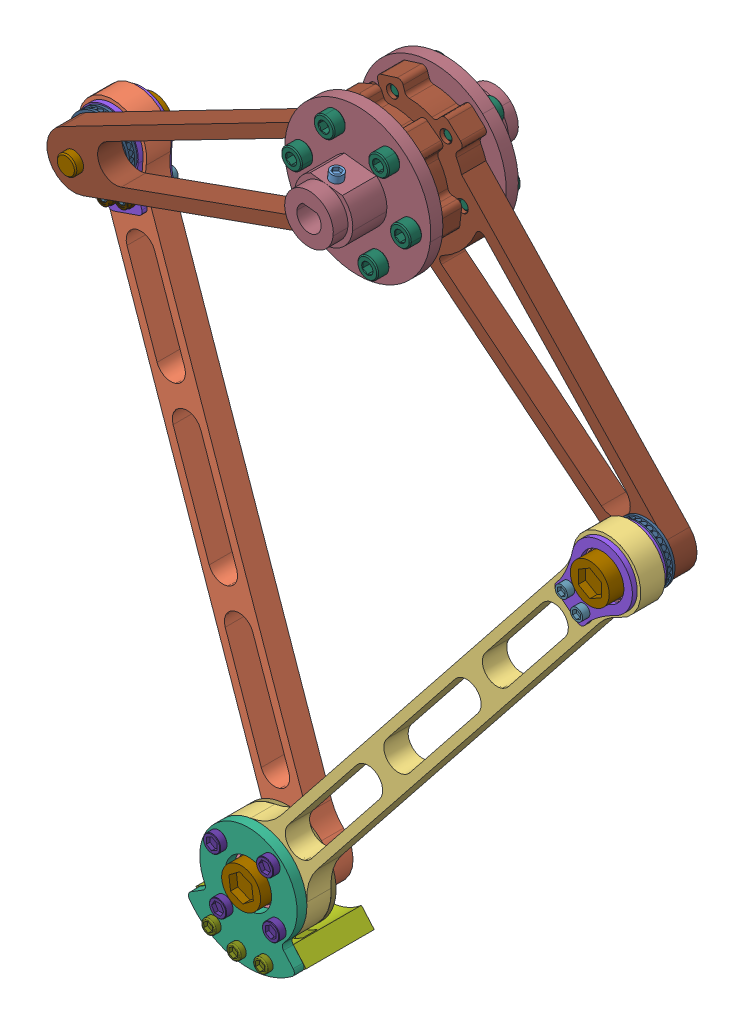
SolidWorks assembly B【部分装配】单腿, configuration 默认. Lengths in mm.
Overall size (272.8 367.82 76).
59 component instances, 19 part files, 123 mates.
Components (placement in the parent):
- 【光杆】M8-26-1: 【光杆】M8-26 [默认] at (-54.1395 107.9451 129.2539) x (0.99429 0.106711 0) z (0 0 1) size (8 8 26)
- 【铝合金结构件】小腿1-1: 【铝合金结构件】小腿1 [默认] at (-175.7689 55.1337 129.2539) x (0.329361 -0.944204 0) z (0 0 1) size (257 28 10)
- 【铝合金结构件】小腿2-1: 【铝合金结构件】小腿2 [默认] at (43.2186 17.9219 145.2539) x (-0.622759 -0.782414 0) z (0 0 1) size (264 40 10)
- 【深沟球轴承】6800ZZ 尺寸：10-19-5-3: 【深沟球轴承】6800ZZ 尺寸：10-19-5 [默认] at (43.2186 17.9219 145.2539) x (0.672447 0.740145 0) z (0 0 1) size (19 19 5)
- 【深沟球轴承】6800ZZ 尺寸：10-19-5-4: 【深沟球轴承】6800ZZ 尺寸：10-19-5 [默认] at (43.2186 17.9219 150.2539) x (1 0.000049 0) z (0 0 1) size (19 19 5)
- 【深沟球轴承】6800ZZ 尺寸：10-19-5-8: 【深沟球轴承】6800ZZ 尺寸：10-19-5 [默认] at (-175.7689 55.1337 134.2539) x (1 -0.000082 0) z (0 0 1) size (19 19 5)
- 【深沟球轴承】6800ZZ 尺寸：10-19-5-9: 【深沟球轴承】6800ZZ 尺寸：10-19-5 [默认] at (-175.7689 55.1337 129.2539) size (19 19 5)
- 【深沟球轴承】6800ZZ 尺寸：10-19-5-10: 【深沟球轴承】6800ZZ 尺寸：10-19-5 [默认] at (-100.016 -162.0332 150.2539) x (1 -0.000016 0) z (0 0 1) size (19 19 5)
- 【深沟球轴承】6800ZZ 尺寸：10-19-5-11: 【深沟球轴承】6800ZZ 尺寸：10-19-5 [默认] at (-100.016 -162.0332 145.2539) x (1 -0.00012 0) z (0 0 1) size (19 19 5)
- 【深沟球轴承】608ZZ 尺寸：8-22-7-3: 【深沟球轴承】608ZZ 尺寸：8-22-7 [Défaut] at (-54.1395 107.9451 151.7539) size (22 22 7)
- 【深沟球轴承】608ZZ 尺寸：8-22-7-4: 【深沟球轴承】608ZZ 尺寸：8-22-7 [Défaut] at (-54.1395 107.9451 132.6539) size (22 22 7)
- 【马蹄结构件】蹄子侧板-3: 【马蹄结构件】蹄子侧板 [默认] at (25.2358 10.7897 159.2539) x (-0.98897 0.148118 0) z (0 0 -1) size (43.97 50 4)
- 【马蹄结构件】蹄子底板-1: 【马蹄结构件】蹄子底板 [默认] at (-169.1792 40.0334 155.2539) x (0.98897 -0.148118 0) z (0 0 1) size (45.72 15.8 28)
- 【碳纤维板垫圈】15-23-1-1: 【碳纤维板垫圈】15-23-1 [默认] at (-175.7689 55.1337 128.2539) x (-0.329361 0.944204 0) z (0 0 1) size (35.5 25 2)
- 【碳纤维板垫圈】15-23-1-3: 【碳纤维板垫圈】15-23-1 [默认] at (-175.7689 55.1337 140.2539) x (-0.329361 0.944204 0) z (0 0 1) size (35.5 25 2)
- 【碳纤维板垫圈】15-23-1-4: 【碳纤维板垫圈】15-23-1 [默认] at (43.2186 17.9219 156.2539) x (0.622759 0.782414 0) z (0 0 1) size (35.5 25 2)
- 【碳纤维板垫圈】15-23-1-5: 【碳纤维板垫圈】15-23-1 [默认] at (43.2186 17.9219 144.2539) x (0.622759 0.782414 0) z (0 0 1) size (35.5 25 2)
- 【塞打螺丝】M10-16-8: 【塞打螺丝】M10-16 [默认] at (-175.7689 55.1337 145.2539) x (1 0 0) z (0 0 -1) size (16 16 36.25)
- 【平面推力滚针轴承】尺寸：10-24-4-7: 【平面推力滚针轴承】尺寸：10-24-4 [默认] at (-175.7689 55.1337 141.2539) size (24 24 4)
- 【铝合金结构件】大腿-6: 【铝合金结构件】大腿 [默认] at (-188.126 -167.5744 109.2539) x (0.744298 -0.667848 0) z (0 0 1) size (92.95 159.3 10)
- 【塞打螺丝】M10-16-9: 【塞打螺丝】M10-16 [默认] at (43.2186 17.9219 139.2539) size (16 16 36.25)
- 【平面推力滚针轴承】尺寸：10-24-4-8: 【平面推力滚针轴承】尺寸：10-24-4 [默认] at (43.2186 17.9219 139.2539) size (24 24 4)
- 【铝合金结构件】大腿-7: 【铝合金结构件】大腿 [默认] at (252.0136 96.3837 93.2539) x (0.311173 0.950353 0) z (0 0 1) size (92.95 159.3 10)
- 【碳纤维板垫圈】17-40-2-2: 【碳纤维板垫圈】17-40-2 [默认] at (-100.016 -162.0332 143.2539) x (0.622759 0.782414 0) z (0 0 1) size (40 40 2)
- 【平面推力滚针轴承】尺寸：10-24-4-9: 【平面推力滚针轴承】尺寸：10-24-4 [默认] at (-100.016 -162.0332 139.2539) size (24 24 4)
- 【塞打螺丝】M10-16-10: 【塞打螺丝】M10-16 [默认] at (-100.016 -162.0332 139.2539) x (-0.606643 0.794975 0) z (0 0 1) size (16 16 36.25)
- 【法兰联轴器】M10-孔3-1: 【法兰联轴器】M10-孔3 [默认] at (-17.0813 108.8956 37.7039) x (0.999235 0.039114 0) z (0 0 1) size (84.85 84.85 25)
  - 3508__________.STEP-1: 3508__________.STEP [默认] at (-37.067 0.4997 66.55) x (-0.707107 -0.707107 0) z (0 0 1) size (60 60 25)
- 【法兰联轴器】M10-孔3-2: 【法兰联轴器】M10-孔3 [默认] at (-82.8494 84.4941 246.8039) x (-0.78293 -0.62211 0) z (0 0 -1) size (84.85 84.85 25)
  - 3508__________.STEP-1: 3508__________.STEP [默认] at (-37.067 0.4997 66.55) x (-0.707107 -0.707107 0) z (0 0 1) size (60 60 25)
- 【螺丝】M3-18 杯头内六角-1: 【螺丝】M3-18 杯头内六角 [默认] at (-173.9466 37.7648 145.2539) x (-1 0 0) z (0 0 -1) size (5 5 21)
- 【螺丝】M3-18 杯头内六角-3: 【螺丝】M3-18 杯头内六角 [默认] at (-166.393 40.3997 145.2539) x (-1 0 0) z (0 0 -1) size (5 5 21)
- 【螺丝】M3-18 杯头内六角-4: 【螺丝】M3-18 杯头内六角 [默认] at (29.502 7.1119 139.2539) size (5 5 21)
- 【螺丝】M3-18 杯头内六角-5: 【螺丝】M3-18 杯头内六角 [默认] at (35.7614 2.1298 139.2539) size (5 5 21)
- 【螺丝】M5-14 杯头内六角-7: 【螺丝】M5-14 杯头内六角 [默认] at (-63.1007 128.5835 146.2539) x (0.012208 0.999925 0) z (0 0 -1) size (8.5 8.5 19)
- 【螺丝】M5-14 杯头内六角-8: 【螺丝】M5-14 杯头内六角 [默认] at (-76.4935 110.5037 146.2539) x (-0.996991 0.07752 0) z (0 0 -1) size (8.5 8.5 19)
- 【螺丝】M5-14 杯头内六角-9: 【螺丝】M5-14 杯头内六角 [默认] at (-67.5323 89.8652 146.2539) x (-0.56563 -0.824659 0) z (0 0 -1) size (8.5 8.5 19)
- 【螺丝】M5-14 杯头内六角-10: 【螺丝】M5-14 杯头内六角 [默认] at (-45.1783 87.3066 146.2539) x (0.431361 -0.902179 0) z (0 0 -1) size (8.5 8.5 19)
- 【螺丝】M5-14 杯头内六角-11: 【螺丝】M5-14 杯头内六角 [默认] at (-31.7854 105.3864 146.2539) x (0.996991 -0.07752 0) z (0 0 -1) size (8.5 8.5 19)
- 【螺丝】M5-14 杯头内六角-12: 【螺丝】M5-14 杯头内六角 [默认] at (-40.7466 126.0249 146.2539) x (0.56563 0.824659 0) z (0 0 -1) size (8.5 8.5 19)
- 【螺丝】M4-14 杯头内六角-1: 【螺丝】M4-14 杯头内六角 [默认] at (-114.097 -183.2929 146.2539) x (0.999786 0.020673 0) z (0 0 1) size (5.77 5.77 15.5)
- 【螺丝】M4-14 杯头内六角-2: 【螺丝】M4-14 杯头内六角 [默认] at (-103.793 -187.252 146.2539) size (5.77 5.77 15.5)
- 【螺丝】M4-14 杯头内六角-3: 【螺丝】M4-14 杯头内六角 [默认] at (-92.7812 -186.4854 146.2539) size (5.77 5.77 15.5)
- 【螺丝】M4-16 杯头内六角-2: 【螺丝】M4-16 杯头内六角 [默认] at (-112.1434 -152.3805 143.2539) size (7.06 7.06 19)
- 【螺丝】M4-16 杯头内六角-5: 【螺丝】M4-16 杯头内六角 [默认] at (-90.3632 -149.9058 143.2539) x (0 -1 0) z (0 0 1) size (7.06 7.06 19)
- 【螺丝】M4-16 杯头内六角-4: 【螺丝】M4-16 杯头内六角 [默认] at (-87.8886 -171.686 143.2539) x (-1 0 0) z (0 0 1) size (7.06 7.06 19)
- 【螺丝】M4-16 杯头内六角-3: 【螺丝】M4-16 杯头内六角 [默认] at (-109.6688 -174.1606 143.2539) x (0 1 0) z (0 0 1) size (7.06 7.06 19)
- 【螺丝】M5-14 杯头内六角-1: 【螺丝】M5-14 杯头内六角 [默认] at (-38.864 124.4651 138.2539) x (0.999993 0.003661 0) z (0 0 1) size (8.5 8.5 19)
- 【螺丝】M5-14 杯头内六角-6: 【螺丝】M5-14 杯头内六角 [默认] at (-60.8085 129.434 138.2539) x (0.5 0.866025 0) z (0 0 1) size (8.5 8.5 19)
- 【螺丝】M5-14 杯头内六角-5: 【螺丝】M5-14 杯头内六角 [默认] at (-76.0839 112.9139 138.2539) x (-0.5 0.866025 0) z (0 0 1) size (8.5 8.5 19)
- 【螺丝】M5-14 杯头内六角-4: 【螺丝】M5-14 杯头内六角 [默认] at (-69.4149 91.425 138.2539) x (-1 0 0) z (0 0 1) size (8.5 8.5 19)
- 【螺丝】M5-14 杯头内六角-3: 【螺丝】M5-14 杯头内六角 [默认] at (-47.4704 86.4561 138.2539) x (-0.5 -0.866025 0) z (0 0 1) size (8.5 8.5 19)
- 【螺丝】M5-14 杯头内六角-2: 【螺丝】M5-14 杯头内六角 [默认] at (-32.195 102.9762 138.2539) x (0.5 -0.866025 0) z (0 0 1) size (8.5 8.5 19)
- 【螺母】M3-4.0 自锁六角螺母 -1: 【螺母】M3-4.0 自锁六角螺母  [默认] at (-173.9466 37.7648 141.2539) size (6.35 5.5 4)
- 【螺母】M3-4.0 自锁六角螺母 -2: 【螺母】M3-4.0 自锁六角螺母  [默认] at (-166.393 40.3997 141.2539) size (6.35 5.5 4)
- 【螺母】M3-4.0 自锁六角螺母 -3: 【螺母】M3-4.0 自锁六角螺母  [默认] at (35.7614 2.1298 143.2539) x (-0.923728 -0.383049 0) z (0 0 -1) size (6.35 5.5 4)
- 【螺母】M3-4.0 自锁六角螺母 -4: 【螺母】M3-4.0 自锁六角螺母  [默认] at (29.502 7.1119 143.2539) x (-0.923728 -0.383049 0) z (0 0 -1) size (6.35 5.5 4)
- 【螺丝】M3-10 杯头内六角-1: 【螺丝】M3-10 杯头内六角 [默认] at (-54.1395 107.9451 170.2539) x (-0.809906 0.092701 -0.579188) z (0.113716 0.993513 0) size (5 5 13)
- 【螺丝】M3-10 杯头内六角-2: 【螺丝】M3-10 杯头内六角 [默认] at (-54.1395 107.9451 114.2539) x (-0.015394 -0.016648 -0.999743) z (-0.734224 0.678908 0) size (5 5 13)
Mates (geometry in assembly coordinates):
- 同心76: concentric: cylinder of assembly; cylinder of assembly; cylinder of 【深沟球轴承】6800ZZ 尺寸：10-19-5-3 through (43.2186 17.9219 150.2539) axis (0 0 -1) radius 5; cylinder of 【深沟球轴承】6800ZZ 尺寸：10-19-5-4 through (43.2186 17.9219 155.2539) axis (0 0 -1) radius 9.5
- 重合56: coincident: plane of assembly; plane of assembly; plane of 【深沟球轴承】6800ZZ 尺寸：10-19-5-4 through (43.2186 17.9219 155.2539) normal (0 0 1); plane of 【铝合金结构件】小腿2-1 through (43.2186 17.9219 155.2539) normal (0 0 1)
- 重合57: coincident: plane of assembly; plane of assembly; plane of 【深沟球轴承】6800ZZ 尺寸：10-19-5-3 through (43.2186 17.9219 145.2539) normal (0 0 -1); plane of 【铝合金结构件】小腿2-1 through (43.2186 17.9219 145.2539) normal (0 0 -1)
- 同心119: concentric: cylinder of assembly; cylinder of assembly; cylinder of 【铝合金结构件】小腿1-1 through (-175.7689 55.1337 139.2539) axis (0 0 -1) radius 9.5; cylinder of 【深沟球轴承】6800ZZ 尺寸：10-19-5-8 through (-175.7689 55.1337 139.2539) axis (0 0 -1) radius 5
- 重合97: coincident: plane of assembly; plane of assembly; plane of 【铝合金结构件】小腿1-1 through (-175.7689 55.1337 139.2539) normal (0 0 1); plane of 【深沟球轴承】6800ZZ 尺寸：10-19-5-8 through (-175.7689 55.1337 139.2539) normal (0 0 1)
- 同心120: concentric: cylinder of assembly; cylinder of assembly; cylinder of 【铝合金结构件】小腿1-1 through (-175.7689 55.1337 139.2539) axis (0 0 -1) radius 9.5; cylinder of 【深沟球轴承】6800ZZ 尺寸：10-19-5-9 through (-175.7689 55.1337 134.2539) axis (0 0 -1) radius 5
- 重合98: coincident: plane of assembly; plane of assembly; plane of 【铝合金结构件】小腿1-1 through (-175.7689 55.1337 129.2539) normal (0 0 -1); plane of 【深沟球轴承】6800ZZ 尺寸：10-19-5-9 through (-175.7689 55.1337 129.2539) normal (0 0 -1)
- 同心127: concentric: cylinder of assembly; cylinder of assembly; cylinder of 【铝合金结构件】小腿2-1 through (-100.016 -162.0332 155.2539) axis (0 0 -1) radius 9.5; cylinder of 【深沟球轴承】6800ZZ 尺寸：10-19-5-10 through (-100.016 -162.0332 155.2539) axis (0 0 -1) radius 5
- 重合102: coincident: plane of assembly; plane of assembly; plane of 【铝合金结构件】小腿2-1 through (43.2186 17.9219 155.2539) normal (0 0 1); plane of 【深沟球轴承】6800ZZ 尺寸：10-19-5-10 through (-100.016 -162.0332 155.2539) normal (0 0 1)
- 同心129: concentric: cylinder of assembly; cylinder of assembly; cylinder of 【铝合金结构件】小腿2-1 through (-100.016 -162.0332 155.2539) axis (0 0 -1) radius 9.5; cylinder of 【深沟球轴承】6800ZZ 尺寸：10-19-5-11 through (-100.016 -162.0332 150.2539) axis (0 0 -1) radius 5
- 重合104: coincident: plane of assembly; plane of assembly; plane of 【铝合金结构件】小腿2-1 through (43.2186 17.9219 145.2539) normal (0 0 -1); plane of 【深沟球轴承】6800ZZ 尺寸：10-19-5-11 through (-100.016 -162.0332 145.2539) normal (0 0 -1)
- 同心159: concentric: cylinder of assembly; cylinder of assembly; cylinder of 【深沟球轴承】608ZZ 尺寸：8-22-7-3 through (-54.1395 107.9451 386.8041) axis (0 0 1) radius 4; cylinder of 【光杆】M8-26-1 through (-54.1395 107.9451 155.2539) axis (0 0 -1) radius 4
- 同心166: concentric: cylinder of assembly; cylinder of assembly; cylinder of 【铝合金结构件】小腿2-1 through (-90.3632 -149.9058 145.2539) axis (0 0 1) radius 2; cylinder of 【马蹄结构件】蹄子侧板-3 through (-90.3632 -149.9058 155.2539) axis (0 0 1) radius 2
- 同心167: concentric: cylinder of assembly; cylinder of assembly; cylinder of 【铝合金结构件】小腿2-1 through (-112.1434 -152.3805 145.2539) axis (0 0 1) radius 2; cylinder of 【马蹄结构件】蹄子侧板-3 through (-112.1434 -152.3805 155.2539) axis (0 0 1) radius 2
- 同心168: concentric: cylinder of assembly; cylinder of assembly; cylinder of 【马蹄结构件】蹄子侧板-3 through (-92.7812 -186.4854 155.2539) axis (0 0 1) radius 2; cylinder of 【马蹄结构件】蹄子底板-1 through (-92.7812 -186.4854 159.2539) axis (0 0 -1) radius 2
- 重合124: coincident: plane of assembly; plane of assembly; plane of 【马蹄结构件】蹄子侧板-3 through (-100.016 -162.0332 155.2539) normal (0 0 -1); plane of 【马蹄结构件】蹄子底板-1 through (-61.4897 -147.4543 155.2539) normal (0 0 1)
- 平行2: parallel: plane of assembly; plane of assembly; plane of 【马蹄结构件】蹄子侧板-3 through (-117.0067 -172.5838 155.2539) normal (-0.52753 0.849536 0); plane of 【马蹄结构件】蹄子底板-1 through (-118.7448 -173.507 127.2539) normal (-0.52753 0.849536 0)
- 同心169: concentric: cylinder of assembly; cylinder of assembly; cylinder of 【深沟球轴承】6800ZZ 尺寸：10-19-5-9 through (-175.7689 55.1337 134.2539) axis (0 0 -1) radius 5; cylinder of 【碳纤维板垫圈】15-23-1-1 through (-175.7689 55.1337 129.2539) axis (0 0 -1) radius 9
- 重合125: coincident: plane of assembly; plane of assembly; plane of 【铝合金结构件】小腿1-1 through (-175.7689 55.1337 129.2539) normal (0 0 -1); plane of 【碳纤维板垫圈】15-23-1-1 through (-175.7689 55.1337 129.2539) normal (0 0 1)
- 同心172: concentric: cylinder of assembly; cylinder of assembly; cylinder of 【深沟球轴承】6800ZZ 尺寸：10-19-5-9 through (-175.7689 55.1337 134.2539) axis (0 0 -1) radius 5; cylinder of 【塞打螺丝】M10-16-8 through (-175.7689 55.1337 129.2539) axis (0 0 1) radius 5
- 重合126: coincident: plane of assembly; plane of assembly; plane of 【深沟球轴承】6800ZZ 尺寸：10-19-5-9 through (-175.7689 55.1337 129.2539) normal (0 0 -1); plane of 【塞打螺丝】M10-16-8 through (-175.7689 55.1337 129.2539) normal (0 0 1)
- 同心177: concentric: cylinder of assembly; cylinder of assembly; cylinder of 【塞打螺丝】M10-16-8 through (-175.7689 55.1337 129.2539) axis (0 0 1) radius 5; cylinder of 【碳纤维板垫圈】15-23-1-3 through (-175.7689 55.1337 141.2539) axis (0 0 -1) radius 9
- 重合130: coincident: plane of assembly; plane of assembly; plane of 【铝合金结构件】小腿1-1 through (-175.7689 55.1337 139.2539) normal (0 0 1); plane of 【碳纤维板垫圈】15-23-1-3 through (-211.4327 18.7427 139.2539) normal (0 0 -1)
- 同心179: concentric: cylinder of assembly; cylinder of assembly; cylinder of 【塞打螺丝】M10-16-8 through (-175.7689 55.1337 158.5039) axis (0 0 -1) radius 4; cylinder of 【平面推力滚针轴承】尺寸：10-24-4-7 through (-175.7689 55.1337 145.2539) axis (0 0 -1) radius 5
- 重合131: coincident: plane of assembly; plane of assembly; plane of 【碳纤维板垫圈】15-23-1-3 through (-175.7689 55.1337 141.2539) normal (0 0 1); plane of 【平面推力滚针轴承】尺寸：10-24-4-7 through (-175.7689 55.1337 141.2539) normal (0 0 -1)
- 同心180: concentric: cylinder of assembly; cylinder of assembly; cylinder of 【塞打螺丝】M10-16-8 through (-175.7689 55.1337 158.5039) axis (0 0 -1) radius 4; cylinder of 【铝合金结构件】大腿-6 through (-175.7689 55.1337 155.2539) axis (0 0 -1) radius 4
- 重合132: coincident: plane of assembly; plane of assembly; plane of 【平面推力滚针轴承】尺寸：10-24-4-7 through (-175.7689 55.1337 145.2539) normal (0 0 1); plane of 【铝合金结构件】大腿-6 through (-54.1395 107.9451 145.2539) normal (0 0 -1)
- 同心183: concentric: cylinder of assembly; cylinder of assembly; cylinder of 【光杆】M8-26-1 through (-54.1395 107.9451 155.2539) axis (0 0 -1) radius 4; cylinder of 【铝合金结构件】大腿-6 through (-54.1395 107.9451 155.2539) axis (0 0 -1) radius 11.05
- 同心184: concentric: cylinder of assembly; cylinder of assembly; cylinder of 【深沟球轴承】6800ZZ 尺寸：10-19-5-4 through (43.2186 17.9219 155.2539) axis (0 0 -1) radius 5; cylinder of 【碳纤维板垫圈】15-23-1-4 through (43.2186 17.9219 157.2539) axis (0 0 -1) radius 9
- 重合134: coincident: plane of assembly; plane of assembly; plane of 【铝合金结构件】小腿2-1 through (43.2186 17.9219 155.2539) normal (0 0 1); plane of 【碳纤维板垫圈】15-23-1-4 through (-6.5894 28.6631 155.2539) normal (0 0 -1)
- 重合135: coincident: plane of assembly; plane of assembly; plane of 【铝合金结构件】小腿2-1 through (43.2186 17.9219 145.2539) normal (0 0 -1); plane of 【碳纤维板垫圈】15-23-1-5 through (43.2186 17.9219 145.2539) normal (0 0 1)
- 同心187: concentric: cylinder of assembly; cylinder of assembly; cylinder of 【深沟球轴承】6800ZZ 尺寸：10-19-5-3 through (43.2186 17.9219 150.2539) axis (0 0 -1) radius 5; cylinder of 【碳纤维板垫圈】15-23-1-5 through (43.2186 17.9219 145.2539) axis (0 0 -1) radius 9
- 同心189: concentric: cylinder of 【深沟球轴承】6800ZZ 尺寸：10-19-5-4 through (43.2186 17.9219 155.2539) axis (0 0 -1) radius 5; cylinder of ? through (43.2186 17.9219 155.2539) axis (0 0 -1) radius 5
- 重合137: coincident: plane of 【深沟球轴承】6800ZZ 尺寸：10-19-5-4 through (43.2186 17.9219 155.2539) normal (0 0 1); plane of ? through (43.2186 17.9219 155.2539) normal (0 0 -1)
- 同心190: concentric: cylinder of ? through (43.2186 17.9219 155.2539) axis (0 0 -1) radius 5; cylinder of ? through (43.2186 17.9219 143.2539) axis (0 0 -1) radius 5
- 重合138: coincident: plane of 【碳纤维板垫圈】15-23-1-5 through (-6.5894 28.6631 143.2539) normal (0 0 -1); plane of ? through (43.2186 17.9219 143.2539) normal (0 0 1)
- 同心192: concentric: cylinder of ? through (43.2186 17.9219 126.0039) axis (0 0 1) radius 4; cylinder of 【铝合金结构件】大腿-7 through (43.2186 17.9219 139.2539) axis (0 0 -1) radius 4
- 重合139: coincident: plane of ? through (43.2186 17.9219 139.2539) normal (0 0 -1); plane of 【铝合金结构件】大腿-7 through (-54.1395 107.9451 139.2539) normal (0 0 1)
- 重合140: coincident: plane of assembly; plane of assembly; plane of 【铝合金结构件】小腿2-1 through (43.2186 17.9219 145.2539) normal (0 0 -1); plane of 【碳纤维板垫圈】17-40-2-2 through (-100.016 -162.0332 145.2539) normal (0 0 1)
- 同心193: concentric: cylinder of assembly; cylinder of assembly; cylinder of 【深沟球轴承】6800ZZ 尺寸：10-19-5-11 through (-100.016 -162.0332 150.2539) axis (0 0 -1) radius 5; cylinder of 【碳纤维板垫圈】17-40-2-2 through (-100.016 -162.0332 145.2539) axis (0 0 -1) radius 8.5
- 同心194: concentric: cylinder of assembly; cylinder of assembly; cylinder of 【铝合金结构件】小腿2-1 through (-90.3632 -149.9058 145.2539) axis (0 0 1) radius 2; cylinder of 【碳纤维板垫圈】17-40-2-2 through (-90.3632 -149.9058 145.2539) axis (0 0 -1) radius 2
- 重合144: coincident: plane of assembly; plane of assembly; plane of 【碳纤维板垫圈】17-40-2-2 through (-100.016 -162.0332 143.2539) normal (0 0 -1); plane of 【平面推力滚针轴承】尺寸：10-24-4-9 through (-100.016 -162.0332 143.2539) normal (0 0 1)
- 同心196: concentric: cylinder of assembly; cylinder of assembly; cylinder of 【碳纤维板垫圈】17-40-2-2 through (-100.016 -162.0332 145.2539) axis (0 0 -1) radius 8.5; cylinder of 【平面推力滚针轴承】尺寸：10-24-4-9 through (-100.016 -162.0332 143.2539) axis (0 0 -1) radius 5
- 重合145: coincident: plane of assembly; plane of assembly; plane of 【铝合金结构件】小腿1-1 through (-175.7689 55.1337 139.2539) normal (0 0 1); plane of 【平面推力滚针轴承】尺寸：10-24-4-9 through (-100.016 -162.0332 139.2539) normal (0 0 -1)
- 同心197: concentric: cylinder of assembly; cylinder of assembly; cylinder of 【铝合金结构件】小腿1-1 through (-100.016 -162.0332 129.2539) axis (0 0 1) radius 4; cylinder of 【平面推力滚针轴承】尺寸：10-24-4-9 through (-100.016 -162.0332 143.2539) axis (0 0 -1) radius 5
- 重合146: coincident: plane of assembly; plane of assembly; plane of 【铝合金结构件】小腿2-1 through (43.2186 17.9219 155.2539) normal (0 0 1); plane of 【马蹄结构件】蹄子侧板-3 through (-100.016 -162.0332 155.2539) normal (0 0 -1)
- 同心200: concentric: cylinder of assembly; cylinder of assembly; cylinder of 【深沟球轴承】6800ZZ 尺寸：10-19-5-10 through (-100.016 -162.0332 155.2539) axis (0 0 -1) radius 5; cylinder of 【塞打螺丝】M10-16-10 through (-100.016 -162.0332 155.2539) axis (0 0 -1) radius 5
- 重合149: coincident: plane of assembly; plane of assembly; plane of 【深沟球轴承】6800ZZ 尺寸：10-19-5-10 through (-100.016 -162.0332 155.2539) normal (0 0 1); plane of 【塞打螺丝】M10-16-10 through (-100.016 -162.0332 155.2539) normal (0 0 -1)
- 同心201: concentric: cylinder of assembly; cylinder of assembly; cylinder of 【铝合金结构件】大腿-6 through (-54.1395 107.9451 155.2539) axis (0 0 -1) radius 11.05; cylinder of 【铝合金结构件】大腿-7 through (-54.1395 107.9451 139.2539) axis (0 0 -1) radius 11.05
- 同心202: concentric: cylinder of assembly; cylinder of assembly; cylinder of 【深沟球轴承】608ZZ 尺寸：8-22-7-3 through (-54.1395 107.9451 386.8041) axis (0 0 1) radius 11; cylinder of 【铝合金结构件】大腿-6 through (-54.1395 107.9451 155.2539) axis (0 0 -1) radius 11.05
- 重合150: coincident: plane of assembly; plane of assembly; plane of 【深沟球轴承】608ZZ 尺寸：8-22-7-3 through (-54.1395 107.9451 155.2539) normal (0 0 1); plane of 【铝合金结构件】大腿-6 through (-54.1395 107.9451 155.2539) normal (0 0 1)
- 同心203: concentric: cylinder of assembly; cylinder of assembly; cylinder of 【铝合金结构件】大腿-7 through (-54.1395 107.9451 139.2539) axis (0 0 -1) radius 11.05; cylinder of 【深沟球轴承】608ZZ 尺寸：8-22-7-4 through (-54.1395 107.9451 367.7041) axis (0 0 1) radius 4
- 重合151: coincident: plane of assembly; plane of assembly; plane of 【铝合金结构件】大腿-7 through (-54.1395 107.9451 129.2539) normal (0 0 -1); plane of 【深沟球轴承】608ZZ 尺寸：8-22-7-4 through (-54.1395 113.8951 129.2539) normal (0 0 -1)
- 重合152: coincident: plane of assembly; plane of assembly; plane of 【深沟球轴承】608ZZ 尺寸：8-22-7-3 through (-54.1395 107.9451 155.2539) normal (0 0 1); plane of 【光杆】M8-26-1 through (-54.1395 107.9451 155.2539) normal (0 0 1)
- 同心204: concentric: cylinder of assembly; cylinder of assembly; cylinder of 【铝合金结构件】小腿1-1 through (-173.9466 37.7648 129.2539) axis (0 0 1) radius 1.5; cylinder of 【碳纤维板垫圈】15-23-1-1 through (-173.9466 37.7648 129.2539) axis (0 0 -1) radius 1.5
- 同心205: concentric: cylinder of assembly; cylinder of assembly; cylinder of 【铝合金结构件】小腿1-1 through (-166.393 40.3997 129.2539) axis (0 0 1) radius 1.5; cylinder of 【碳纤维板垫圈】15-23-1-3 through (-166.393 40.3997 141.2539) axis (0 0 -1) radius 1.5
- 同心206: concentric: cylinder of assembly; cylinder of assembly; cylinder of 【铝合金结构件】小腿2-1 through (43.2186 17.9219 155.2539) axis (0 0 -1) radius 9.5; cylinder of 【深沟球轴承】6800ZZ 尺寸：10-19-5-4 through (43.2186 17.9219 155.2539) axis (0 0 -1) radius 9.5
- 同心207: concentric: cylinder of assembly; cylinder of assembly; cylinder of 【铝合金结构件】小腿2-1 through (35.7614 2.1298 145.2539) axis (0 0 1) radius 1.5; cylinder of 【碳纤维板垫圈】15-23-1-4 through (35.7614 2.1298 157.2539) axis (0 0 -1) radius 1.5
- 同心208: concentric: cylinder of assembly; cylinder of assembly; cylinder of 【铝合金结构件】小腿2-1 through (29.502 7.1119 145.2539) axis (0 0 1) radius 1.5; cylinder of 【碳纤维板垫圈】15-23-1-5 through (29.502 7.1119 145.2539) axis (0 0 -1) radius 1.5
- 同心212: concentric: cylinder of ? through (-54.1395 107.9451 139.2539) axis (0 0 -1) radius 22.5; cylinder of ? through (-54.1395 107.9451 129.2539) axis (0 0 -1) radius 30
- 重合156: coincident: plane of ? through (-54.1395 107.9451 129.2539) normal (0 0 -1); plane of ? through (-54.1395 107.9451 129.2539) normal (0 0 1)
- 同心214: concentric: cylinder of ? through (-61.2587 129.2891 139.2539) axis (0 0 -1) radius 2.5; cylinder of ? through (-61.2587 129.2891 129.2539) axis (0 0 -1) radius 2.5
- 同心215: concentric: cylinder of ? through (-54.1395 107.9451 155.2539) axis (0 0 -1) radius 22.5; cylinder of ? through (-54.1395 107.9451 155.2539) axis (0 0 1) radius 30
- 重合157: coincident: plane of ? through (-54.1395 107.9451 155.2539) normal (0 0 1); plane of ? through (-54.1395 107.9451 155.2539) normal (0 0 -1)
- 同心216: concentric: cylinder of ? through (-66.2202 126.9268 155.2539) axis (0 0 -1) radius 2.5; cylinder of ? through (-66.2202 126.9268 155.2539) axis (0 0 1) radius 2.5
- 同心217: concentric: cylinder of assembly; cylinder of assembly; cylinder of 【碳纤维板垫圈】15-23-1-1 through (-173.9466 37.7648 129.2539) axis (0 0 -1) radius 1.5; cylinder of 【螺丝】M3-18 杯头内六角-1 through (-173.9466 37.7648 127.2539) axis (0 0 1) radius 1.5
- 重合158: coincident: plane of assembly; plane of assembly; plane of 【碳纤维板垫圈】15-23-1-1 through (-211.4327 18.7427 127.2539) normal (0 0 -1); plane of 【螺丝】M3-18 杯头内六角-1 through (-173.9466 37.7648 127.2539) normal (0 0 1)
- 同心218: concentric: cylinder of assembly; cylinder of assembly; cylinder of 【碳纤维板垫圈】15-23-1-1 through (-166.393 40.3997 129.2539) axis (0 0 -1) radius 1.5; cylinder of 【螺丝】M3-18 杯头内六角-3 through (-166.393 40.3997 127.2539) axis (0 0 1) radius 1.5
- 重合159: coincident: plane of assembly; plane of assembly; plane of 【碳纤维板垫圈】15-23-1-1 through (-211.4327 18.7427 127.2539) normal (0 0 -1); plane of 【螺丝】M3-18 杯头内六角-3 through (-166.393 40.3997 127.2539) normal (0 0 1)
- 同心221: concentric: cylinder of assembly; cylinder of assembly; cylinder of 【碳纤维板垫圈】15-23-1-4 through (29.502 7.1119 157.2539) axis (0 0 -1) radius 1.5; cylinder of 【螺丝】M3-18 杯头内六角-4 through (29.502 7.1119 157.2539) axis (0 0 -1) radius 1.5
- 重合162: coincident: plane of assembly; plane of assembly; plane of 【碳纤维板垫圈】15-23-1-4 through (43.2186 17.9219 157.2539) normal (0 0 1); plane of 【螺丝】M3-18 杯头内六角-4 through (29.502 7.1119 157.2539) normal (0 0 -1)
- 同心222: concentric: cylinder of assembly; cylinder of assembly; cylinder of 【碳纤维板垫圈】15-23-1-4 through (35.7614 2.1298 157.2539) axis (0 0 -1) radius 1.5; cylinder of 【螺丝】M3-18 杯头内六角-5 through (35.7614 2.1298 157.2539) axis (0 0 -1) radius 1.5
- 重合163: coincident: plane of assembly; plane of assembly; plane of 【碳纤维板垫圈】15-23-1-4 through (43.2186 17.9219 157.2539) normal (0 0 1); plane of 【螺丝】M3-18 杯头内六角-5 through (35.7614 2.1298 157.2539) normal (0 0 -1)
- 同心226: concentric: cylinder of ? through (-39.2147 124.7825 129.2539) axis (0 0 -1) radius 2.5; cylinder of ? through (-39.2147 124.7825 119.2539) axis (0 0 1) radius 4.25
- 重合167: coincident: plane of ? through (-54.1395 107.9451 124.2539) normal (0 0 -1); plane of ? through (-39.2147 124.7825 124.2539) normal (0 0 1)
- 同心227: concentric: cylinder of ? through (-66.2202 126.9268 155.2539) axis (0 0 1) radius 2.5; cylinder of ? through (-66.2202 126.9268 165.2539) axis (0 0 -1) radius 4.25
- 重合168: coincident: plane of ? through (-54.1395 107.9451 160.2539) normal (0 0 1); plane of ? through (-66.2202 126.9268 160.2539) normal (0 0 -1)
- 同心228: concentric: cylinder of assembly; cylinder of assembly; cylinder of 【马蹄结构件】蹄子侧板-3 through (-112.1434 -152.3805 155.2539) axis (0 0 1) radius 2; cylinder of 【螺丝】M4-16 杯头内六角-2 through (-112.1434 -152.3805 159.2539) axis (0 0 -1) radius 2
- 重合169: coincident: plane of assembly; plane of assembly; plane of 【马蹄结构件】蹄子侧板-3 through (-100.016 -162.0332 159.2539) normal (0 0 1); plane of 【螺丝】M4-16 杯头内六角-2 through (-112.1434 -152.3805 159.2539) normal (0 0 -1)
- 同心230: concentric: cylinder of assembly; cylinder of assembly; cylinder of 【马蹄结构件】蹄子侧板-3 through (-114.097 -183.2929 155.2539) axis (0 0 1) radius 2; cylinder of 【螺丝】M4-14 杯头内六角-1 through (-114.097 -183.2929 159.2539) axis (0 0 -1) radius 2
- 重合170: coincident: plane of assembly; plane of assembly; plane of 【马蹄结构件】蹄子侧板-3 through (-100.016 -162.0332 159.2539) normal (0 0 1); plane of 【螺丝】M4-14 杯头内六角-1 through (-114.097 -183.2929 159.2539) normal (0 0 -1)
- 同心231: concentric: cylinder of assembly; cylinder of assembly; cylinder of 【马蹄结构件】蹄子侧板-3 through (-103.793 -187.252 155.2539) axis (0 0 1) radius 2; cylinder of 【螺丝】M4-14 杯头内六角-2 through (-103.793 -187.252 159.2539) axis (0 0 -1) radius 2
- 重合171: coincident: plane of assembly; plane of assembly; plane of 【马蹄结构件】蹄子侧板-3 through (-100.016 -162.0332 159.2539) normal (0 0 1); plane of 【螺丝】M4-14 杯头内六角-2 through (-103.793 -187.252 159.2539) normal (0 0 -1)
- 同心232: concentric: cylinder of assembly; cylinder of assembly; cylinder of 【马蹄结构件】蹄子侧板-3 through (-92.7812 -186.4854 155.2539) axis (0 0 1) radius 2; cylinder of 【螺丝】M4-14 杯头内六角-3 through (-92.7812 -186.4854 159.2539) axis (0 0 -1) radius 2
- 重合172: coincident: plane of assembly; plane of assembly; plane of 【马蹄结构件】蹄子侧板-3 through (-100.016 -162.0332 159.2539) normal (0 0 1); plane of 【螺丝】M4-14 杯头内六角-3 through (-92.7812 -186.4854 159.2539) normal (0 0 -1)
- 同心233: concentric: cylinder of assembly; cylinder of assembly; cylinder of 【螺丝】M3-18 杯头内六角-5 through (35.7614 2.1298 157.2539) axis (0 0 -1) radius 1.5; cylinder of 【螺母】M3-4.0 自锁六角螺母 -3 through (35.7614 2.1298 142.9767) axis (0 0 -1) radius 1.5
- 同心234: concentric: cylinder of assembly; cylinder of assembly; cylinder of 【螺丝】M3-18 杯头内六角-4 through (29.502 7.1119 157.2539) axis (0 0 -1) radius 1.5; cylinder of 【螺母】M3-4.0 自锁六角螺母 -4 through (29.502 7.1119 142.9767) axis (0 0 -1) radius 1.5
- 重合173: coincident: plane of assembly; plane of assembly; plane of 【碳纤维板垫圈】15-23-1-5 through (-6.5894 28.6631 143.2539) normal (0 0 -1); plane of 【螺母】M3-4.0 自锁六角螺母 -3 through (35.7614 2.1298 143.2539) normal (0 0 1)
- 重合174: coincident: plane of assembly; plane of assembly; plane of 【碳纤维板垫圈】15-23-1-5 through (-6.5894 28.6631 143.2539) normal (0 0 -1); plane of 【螺母】M3-4.0 自锁六角螺母 -4 through (29.502 7.1119 143.2539) normal (0 0 1)
- 重合175: coincident: plane of assembly; plane of assembly; plane of 【碳纤维板垫圈】15-23-1-3 through (-175.7689 55.1337 141.2539) normal (0 0 1); plane of 【螺母】M3-4.0 自锁六角螺母 -1 through (-173.9466 37.7648 141.2539) normal (0 0 -1)
- 同心235: concentric: cylinder of assembly; cylinder of assembly; cylinder of 【螺丝】M3-18 杯头内六角-1 through (-173.9466 37.7648 127.2539) axis (0 0 1) radius 1.5; cylinder of 【螺母】M3-4.0 自锁六角螺母 -1 through (-173.9466 37.7648 141.531) axis (0 0 1) radius 1.5
- 重合176: coincident: plane of assembly; plane of assembly; plane of 【碳纤维板垫圈】15-23-1-3 through (-175.7689 55.1337 141.2539) normal (0 0 1); plane of 【螺母】M3-4.0 自锁六角螺母 -2 through (-166.393 40.3997 141.2539) normal (0 0 -1)
- 同心236: concentric: cylinder of assembly; cylinder of assembly; cylinder of 【螺丝】M3-18 杯头内六角-3 through (-166.393 40.3997 127.2539) axis (0 0 1) radius 1.5; cylinder of 【螺母】M3-4.0 自锁六角螺母 -2 through (-166.393 40.3997 141.531) axis (0 0 1) radius 1.5
- 同心237: concentric: cylinder of 【法兰联轴器】M10-孔3-1/3508__________.STEP-1 through (-57.0764 110.6607 114.2539) axis (0.734224 -0.678908 0) radius 1.5; cylinder of 【螺丝】M3-10 杯头内六角-2 through (-61.4817 114.7341 114.2539) axis (0.734224 -0.678908 0) radius 1.5
- 重合177: coincident: plane of 【法兰联轴器】M10-孔3-1/3508__________.STEP-1 through (-61.4817 114.7341 124.2539) normal (-0.734224 0.678908 0); plane of 【螺丝】M3-10 杯头内六角-2 through (-61.4817 114.7341 114.2539) normal (0.734224 -0.678908 0)
- 同心238: concentric: cylinder of 【法兰联轴器】M10-孔3-2/3508__________.STEP-1 through (-53.6846 111.9191 170.2539) axis (-0.113716 -0.993513 0) radius 1.5; cylinder of 【螺丝】M3-10 杯头内六角-1 through (-53.0023 117.8802 170.2539) axis (-0.113716 -0.993513 0) radius 1.5
- 重合178: coincident: plane of 【法兰联轴器】M10-孔3-2/3508__________.STEP-1 through (-53.0023 117.8802 160.2539) normal (0.113716 0.993513 0); plane of 【螺丝】M3-10 杯头内六角-1 through (-53.0023 117.8802 170.2539) normal (-0.113716 -0.993513 0)
- 同心239: concentric: cylinder of 【法兰联轴器】M10-孔3-2/3508__________.STEP-1 through (-40.7466 126.0249 155.2539) axis (0 0 1) radius 2.5; cylinder of 【螺丝】M5-14 杯头内六角-12 through (-40.7466 126.0249 165.2539) axis (0 0 -1) radius 4.25
- 同心241: concentric: cylinder of 【铝合金结构件】大腿-6 through (-40.7466 126.0249 155.2539) axis (0 0 -1) radius 2.5; cylinder of 【法兰联轴器】M10-孔3-2/3508__________.STEP-1 through (-40.7466 126.0249 155.2539) axis (0 0 1) radius 2.5
- 同心242: concentric: cylinder of assembly; cylinder of assembly; cylinder of 【铝合金结构件】大腿-6 through (-63.1007 128.5835 155.2539) axis (0 0 -1) radius 2.5; cylinder of 【螺丝】M5-14 杯头内六角-7 through (-63.1007 128.5835 165.2539) axis (0 0 -1) radius 4.25
- 重合179: coincident: plane of 【铝合金结构件】大腿-6 through (-54.1395 107.9451 155.2539) normal (0 0 1); plane of 【法兰联轴器】M10-孔3-2/3508__________.STEP-1 through (-54.1395 107.9451 155.2539) normal (0 0 -1)
- 同心243: concentric: cylinder of assembly; cylinder of assembly; cylinder of 【铝合金结构件】大腿-6 through (-63.1007 128.5835 155.2539) axis (0 0 -1) radius 2.5; cylinder of 【螺丝】M5-14 杯头内六角-7 through (-63.1007 128.5835 165.2539) axis (0 0 -1) radius 4.25
- 同心244: concentric: cylinder of 【铝合金结构件】大腿-6 through (-63.1007 128.5835 155.2539) axis (0 0 -1) radius 2.5; cylinder of 【法兰联轴器】M10-孔3-2/3508__________.STEP-1 through (-63.1007 128.5835 155.2539) axis (0 0 1) radius 2.5
- 重合180: coincident: plane of 【法兰联轴器】M10-孔3-2/3508__________.STEP-1 through (-54.1395 107.9451 160.2539) normal (0 0 1); plane of 【螺丝】M5-14 杯头内六角-7 through (-63.1007 128.5835 160.2539) normal (0 0 -1)
- 同心245: concentric: cylinder of 【法兰联轴器】M10-孔3-2/3508__________.STEP-1 through (-31.7854 105.3864 155.2539) axis (0 0 1) radius 2.5; cylinder of 【螺丝】M5-14 杯头内六角-11 through (-31.7854 105.3864 165.2539) axis (0 0 -1) radius 4.25
- 同心246: concentric: cylinder of 【法兰联轴器】M10-孔3-2/3508__________.STEP-1 through (-45.1783 87.3066 155.2539) axis (0 0 1) radius 2.5; cylinder of 【螺丝】M5-14 杯头内六角-10 through (-45.1783 87.3066 165.2539) axis (0 0 -1) radius 4.25
- 同心247: concentric: cylinder of 【法兰联轴器】M10-孔3-2/3508__________.STEP-1 through (-67.5323 89.8652 155.2539) axis (0 0 1) radius 2.5; cylinder of 【螺丝】M5-14 杯头内六角-9 through (-67.5323 89.8652 165.2539) axis (0 0 -1) radius 4.25
- 同心248: concentric: cylinder of 【法兰联轴器】M10-孔3-2/3508__________.STEP-1 through (-76.4935 110.5037 155.2539) axis (0 0 1) radius 2.5; cylinder of 【螺丝】M5-14 杯头内六角-8 through (-76.4935 110.5037 165.2539) axis (0 0 -1) radius 4.25
- 同心249: concentric: cylinder of 【铝合金结构件】大腿-7 through (-38.864 124.4651 139.2539) axis (0 0 -1) radius 2.5; cylinder of 【法兰联轴器】M10-孔3-1/3508__________.STEP-1 through (-38.864 124.4651 129.2539) axis (0 0 -1) radius 2.5
- 同心250: concentric: cylinder of 【铝合金结构件】大腿-7 through (-69.4149 91.425 139.2539) axis (0 0 -1) radius 2.5; cylinder of 【法兰联轴器】M10-孔3-1/3508__________.STEP-1 through (-69.4149 91.425 129.2539) axis (0 0 -1) radius 2.5
- 同心251: concentric: cylinder of 【法兰联轴器】M10-孔3-1/3508__________.STEP-1 through (-47.4704 86.4561 129.2539) axis (0 0 -1) radius 2.5; cylinder of 【螺丝】M5-14 杯头内六角-3 through (-47.4704 86.4561 119.2539) axis (0 0 1) radius 4.25
- 同心252: concentric: cylinder of 【法兰联轴器】M10-孔3-1/3508__________.STEP-1 through (-38.864 124.4651 129.2539) axis (0 0 -1) radius 2.5; cylinder of 【螺丝】M5-14 杯头内六角-1 through (-38.864 124.4651 119.2539) axis (0 0 1) radius 4.25
- 同心253: concentric: cylinder of 【法兰联轴器】M10-孔3-1/3508__________.STEP-1 through (-32.195 102.9762 129.2539) axis (0 0 -1) radius 2.5; cylinder of 【螺丝】M5-14 杯头内六角-2 through (-32.195 102.9762 119.2539) axis (0 0 1) radius 4.25
- 同心254: concentric: cylinder of 【法兰联轴器】M10-孔3-1/3508__________.STEP-1 through (-60.8085 129.434 129.2539) axis (0 0 -1) radius 2.5; cylinder of 【螺丝】M5-14 杯头内六角-6 through (-60.8085 129.434 119.2539) axis (0 0 1) radius 4.25
- 同心255: concentric: cylinder of 【法兰联轴器】M10-孔3-1/3508__________.STEP-1 through (-76.0839 112.9139 129.2539) axis (0 0 -1) radius 2.5; cylinder of 【螺丝】M5-14 杯头内六角-5 through (-76.0839 112.9139 119.2539) axis (0 0 1) radius 4.25
- 同心256: concentric: cylinder of 【法兰联轴器】M10-孔3-1/3508__________.STEP-1 through (-69.4149 91.425 129.2539) axis (0 0 -1) radius 2.5; cylinder of 【螺丝】M5-14 杯头内六角-4 through (-69.4149 91.425 119.2539) axis (0 0 1) radius 4.25
- 重合181: coincident: plane of 【法兰联轴器】M10-孔3-1/3508__________.STEP-1 through (-54.1395 107.9451 124.2539) normal (0 0 -1); plane of 【螺丝】M5-14 杯头内六角-1 through (-38.864 124.4651 124.2539) normal (0 0 1)
- 重合182: coincident: plane of 【法兰联轴器】M10-孔3-1/3508__________.STEP-1 through (-54.1395 107.9451 124.2539) normal (0 0 -1); plane of 【螺丝】M5-14 杯头内六角-6 through (-60.8085 129.434 124.2539) normal (0 0 1)
- 重合183: coincident: plane of 【法兰联轴器】M10-孔3-1/3508__________.STEP-1 through (-54.1395 107.9451 124.2539) normal (0 0 -1); plane of 【螺丝】M5-14 杯头内六角-5 through (-76.0839 112.9139 124.2539) normal (0 0 1)
- 重合184: coincident: plane of 【法兰联轴器】M10-孔3-1/3508__________.STEP-1 through (-54.1395 107.9451 124.2539) normal (0 0 -1); plane of 【螺丝】M5-14 杯头内六角-4 through (-69.4149 91.425 124.2539) normal (0 0 1)
- 重合185: coincident: plane of 【法兰联轴器】M10-孔3-1/3508__________.STEP-1 through (-54.1395 107.9451 124.2539) normal (0 0 -1); plane of 【螺丝】M5-14 杯头内六角-3 through (-47.4704 86.4561 124.2539) normal (0 0 1)
- 重合186: coincident: plane of 【法兰联轴器】M10-孔3-1/3508__________.STEP-1 through (-54.1395 107.9451 124.2539) normal (0 0 -1); plane of 【螺丝】M5-14 杯头内六角-2 through (-32.195 102.9762 124.2539) normal (0 0 1)
- 重合187: coincident: plane of 【铝合金结构件】大腿-7 through (-54.1395 107.9451 129.2539) normal (0 0 -1); plane of 【法兰联轴器】M10-孔3-1/3508__________.STEP-1 through (-54.1395 107.9451 129.2539) normal (0 0 1)
